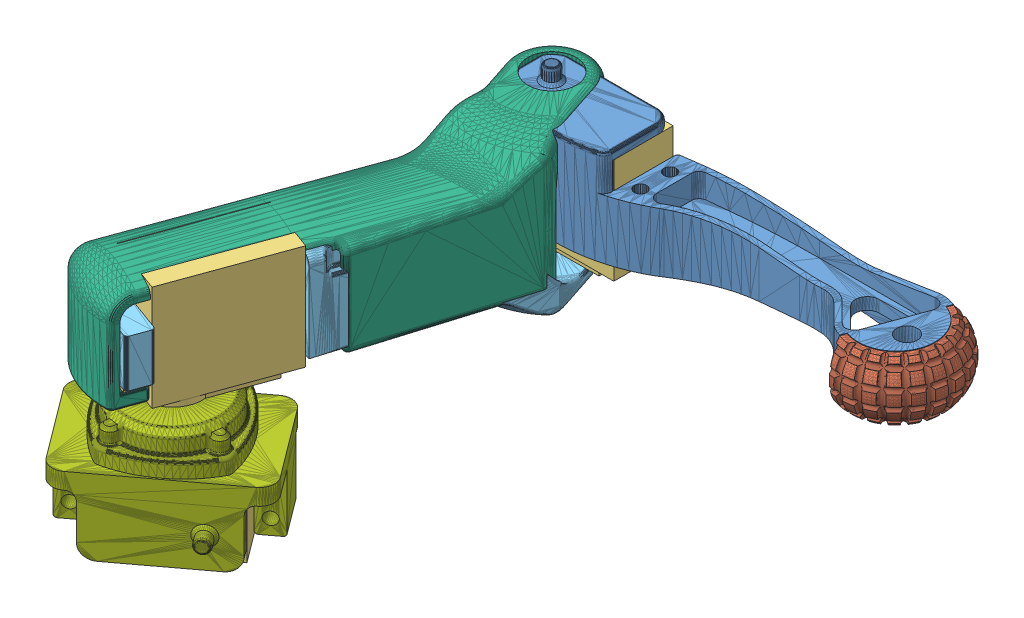
SolidWorks assembly right_foot_back, configuration Default. Lengths in mm.
Overall size (200.98 91.6 160.78).
14 component instances, 7 part files, 20 mates.
Components (placement in the parent):
- R_wrist_mg-1: R_wrist_mg [Default] at (-88.5645 -25.7472 139.9903) size (149.99 36.9 30)
- foot-1: foot [Default] at (37.4355 -5.9472 149.9903) x (0.342021 0 -0.939692) z (-0.939692 0 -0.342021) size (38.32 20 19.41)
- MG996R-1: MG996R [Default] at (-68.3145 3.2528 149.9903) x (1 0 0) z (0 0 -1) size (54.5 43 20)
  - servo-1: servo [Default] at origin size (54.5 39 20)
  - shaft-1: shaft [Default] at (-10.1089 43 0) x (-0.837169 0 -0.546944) z (-0.546944 0 0.837169) size (5.9 19.57 5.9)
- R_arm_mg-1: R_arm_mg [Default] at (-114.624 -85.7472 261.3592) x (0.939851 0 0.341583) z (0.341583 0 -0.939851) size (38.24 39.8 137.4)
- MG996R-2: MG996R [Default] at (-98.3085 -3.7472 245.7431) x (0.341583 0 -0.939851) z (-0.939851 0 -0.341583) size (54.5 43 20)
  - servo-1: servo [Default] at origin size (54.5 39 20)
  - shaft-1: shaft [Default] at (-10.1089 43 0) x (-0.837169 0 -0.546944) z (-0.546944 0 0.837169) size (5.9 19.57 5.9)
- R_arm_cover-1: R_arm_cover [Default] at (-124.4823 -48.0472 265.2243) x (0.939851 0 0.341583) z (0.341583 0 -0.939851) size (41.16 45 143.55)
- MG996R-3: MG996R [Default] at (-92.0933 -70.4472 268.2347) x (-0.80055 0 0.599266) z (0 -1 0) size (54.5 43 20)
  - servo-1: servo [Default] at origin size (54.5 39 20)
  - shaft-1: shaft [Default] at (-10.1089 43 0) x (-0.837169 0 -0.546944) z (-0.546944 0 0.837169) size (5.9 19.57 5.9)
- L_arm_joint_mg-1: L_arm_joint_mg [Default] at (-79.4777 -80.4472 251.2962) x (0 1 0) z (-0.80055 0 0.599266) size (37.5 46 56.5)
Mates (geometry in assembly coordinates):
- Coincident1: coincident anti-aligned: plane of R_wrist_mg-1 through (25.9102 -25.7472 181.6558) normal (0.939692 0 0.342021); plane of foot-1 through (37.4355 -5.9472 149.9903) normal (-0.939692 0 -0.342021)
- Coincident2: coincident anti-aligned: plane of R_wrist_mg-1 through (-88.5645 -8.7472 139.9903) normal (0 1 0); plane of foot-1 through (37.4355 -8.7472 149.9903) normal (0 -1 0)
- Coincident4: coincident: plane of R_wrist_mg-1 through (-84.7772 -25.7472 127.2361) normal (-0.284661 0 0.958628); point of foot-1
- Coincident5: coincident anti-aligned: plane of R_wrist_mg-1 through (-88.5645 3.2528 139.9903) normal (0 -1 0); plane of MG996R-1/servo-1 through (-68.3145 3.2528 149.9903) normal (0 1 0)
- Coincident6: coincident anti-aligned: plane of R_wrist_mg-1 through (-88.5645 -25.7472 139.9903) normal (1 0 0); plane of MG996R-1/servo-1 through (-88.5645 -32.2472 139.9903) normal (-1 0 0)
- Coincident7: coincident anti-aligned: plane of R_wrist_mg-1 through (-88.5645 -25.7472 159.9903) normal (0 0 -1); plane of MG996R-1/servo-1 through (-88.5645 -32.2472 159.9903) normal (0 0 1)
- Parallel1: parallel anti-aligned: plane of R_wrist_mg-1 through (-88.5645 6.1528 139.9903) normal (0 1 0); plane of R_arm_mg-1 through (-114.624 -45.7472 261.3592) normal (0 -1 0)
- Coincident9: coincident: line of MG996R-1/shaft-1 through (-78.4234 -39.7472 149.9903) axis (0 1 0)
- Distance1: distance = 1 mm anti-aligned: plane of MG996R-1/shaft-1 through (-78.4234 -39.7472 149.9903) normal (0 -1 0); plane of R_arm_mg-1 through (-114.624 -40.7472 261.3592) normal (0 1 0)
- Coincident11: coincident anti-aligned: plane of R_arm_mg-1 through (-114.624 -30.7472 261.3592) normal (0 -1 0); plane of MG996R-2/servo-1 through (-102.213 -30.7472 270.392) normal (0 1 0)
- Coincident12: coincident anti-aligned: plane of R_arm_mg-1 through (-100.7899 -85.7472 223.2953) normal (-0.341583 0 0.939851); plane of MG996R-2/servo-1 through (-100.7899 -39.2472 223.2953) normal (0.341583 0 -0.939851)
- Coincident13: coincident anti-aligned: plane of R_arm_mg-1 through (-114.624 -85.7472 261.3592) normal (0.939851 0 0.341583); plane of MG996R-2/servo-1 through (-114.624 -39.2472 261.3592) normal (-0.939851 0 -0.341583)
- Coincident20: coincident anti-aligned: plane of R_arm_cover-1 through (-124.8238 -48.0472 266.1642) normal (0.341583 0 -0.939851); plane of R_arm_mg-1 through (-117.3567 -85.7472 268.878) normal (-0.341583 0 0.939851)
- Coincident21: coincident anti-aligned: plane of MG996R-2/servo-1 through (-102.213 -33.2472 270.392) normal (0 -1 0); plane of R_arm_cover-1 through (-124.4823 -33.2472 265.2243) normal (0 1 0)
- Coincident22: coincident aligned: plane of MG996R-2/servo-1 through (-96.7669 -30.7472 267.8493) normal (0.939851 0 0.341583); plane of R_arm_cover-1 through (-99.158 -48.0472 274.4283) normal (0.939851 0 0.341583)
- Distance2: distance = 1 mm aligned: plane of MG996R-2/shaft-1 through (-101.7615 -46.7472 255.2439) normal (0 -1 0); plane of L_arm_joint_mg-1 through (-79.4777 -45.7472 251.2962) normal (0 -1 0)
- Coincident24: coincident: line of MG996R-2/shaft-1 through (-101.7615 -46.7472 255.2439) axis (0 1 0)
- Coincident26: coincident anti-aligned: plane of MG996R-3/servo-1 through (-97.1561 -60.4472 227.68) normal (0 1 0); plane of L_arm_joint_mg-1 through (-79.4777 -60.4472 251.2962) normal (0 -1 0)
- Coincident27: coincident anti-aligned: plane of MG996R-3/servo-1 through (-129.5784 -80.4472 251.9503) normal (-0.80055 0 0.599266); plane of L_arm_joint_mg-1 through (-111.9 -80.4472 275.5665) normal (0.80055 0 -0.599266)
- Coincident28: coincident anti-aligned: plane of MG996R-3/servo-1 through (-127.8869 -65.6972 261.3018) normal (0.599266 0 0.80055); plane of L_arm_joint_mg-1 through (-92.0623 -80.4472 234.4847) normal (-0.599266 0 -0.80055)
